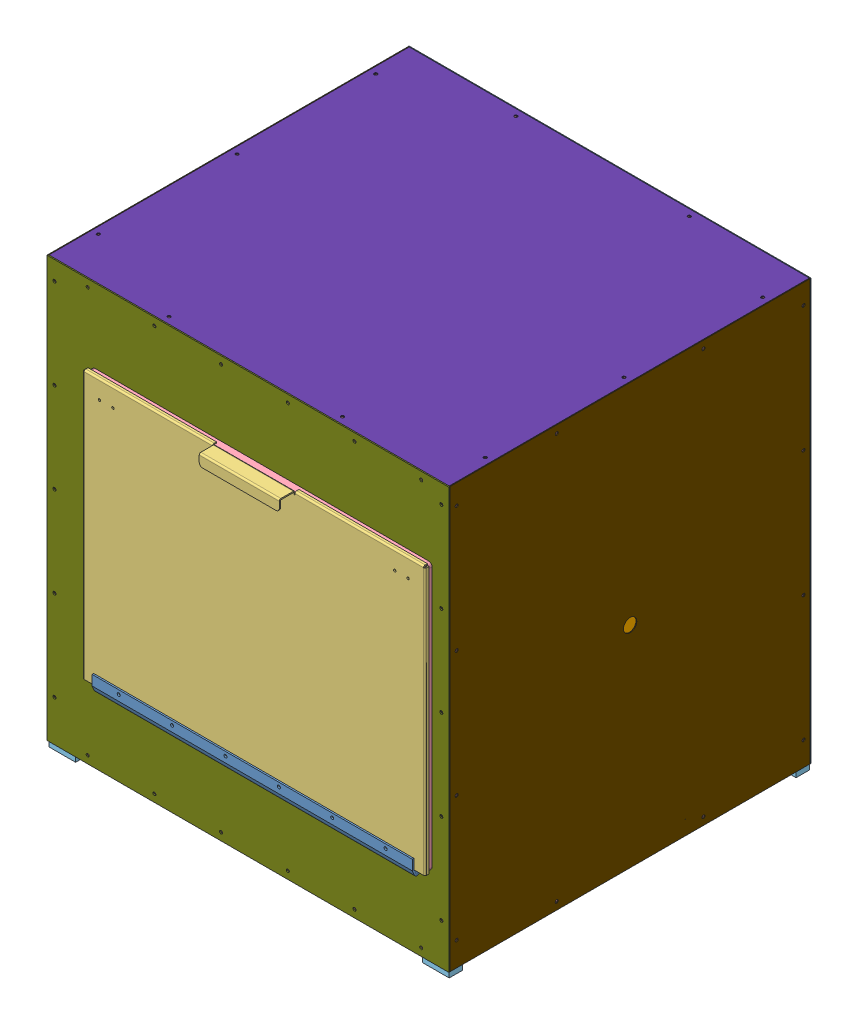
SolidWorks assembly Larva Tracker Assembly_Updated, configuration Default. Lengths in mm.
Overall size (765.17 811.21 817.56).
531 component instances, 63 part files, 154 mates.
Components (placement in the parent):
- T-LSR450-2: T-LSR450 [Default] at (-127.5387 61.5256 -39.6366) x (0 0 -1) z (1 0 0) size (65 43.34 637)
  - NM17-H-1: NM17-H [Default] at (-58.1732 -51.5031 48.5355) size (42.1 42.1 71.3)
  - T-NM17 Housing-1: T-NM17 Housing [Default] at (-16.1232 -51.2531 48.5355) x (-1 0 0) z (0 0 -1) size (41.8 41.8 52)
  - knob_LA-1: knob_LA [Default] at (-37.2232 -26.0531 -6.7645) (suppressed, hidden)
  - Coupling_CPS12-1: Coupling_CPS12 [Default] at (-37.0232 -30.3531 128.8355) x (0.334969 -0.942229 0) z (0 0 -1) size (12 12 14)
  - Car sub assy-1: Car sub assy [Default] at (-37.0232 -30.3531 234.0931) size (64 28.83 65.47) (suppressed, hidden)
    - Lead Screw Nut-1: Lead Screw Nut [Default] at origin size (22.86 20.6 25.4)
    - Screw_M3x12 CS-1: Screw_M3x12 CS [Default] at (8.2532 -4.765 4.546) size (5.92 5.92 12)
    - Screw_M3x12 CS-2: Screw_M3x12 CS [Default] at (-8.2532 -4.765 4.546) size (5.92 5.92 12)
    - Screw_M3x12 CS-3: Screw_M3x12 CS [Default] at (0 9.53 4.546) size (5.92 5.92 12)
    - Washer_5-32ID-1: Washer_5-32ID [Default] at (18.1354 5.1807 -52.75) x (0.633432 -0.633432 -0.44444) z (0.707107 0.707107 0) size (6.35 6.35 0.33)
    - Bearing Washer-1: Bearing Washer [Default] at (-18.3674 -8.3405 -0.25) x (0.5 -0.5 -0.707107) z (0.707107 0.707107 0) size (6.35 6.35 0.2)
    - 3%8 in bearing-1: 3%8 in bearing [Default] at (18.226 -8.199 -0.25) x (0.42856 0.42856 -0.795407) z (-0.707107 0.707107 0) size (9.53 9.53 3.17)
    - Bearing Washer-2: Bearing Washer [Default] at (15.9809 -5.954 -0.25) x (0.5 0.5 0.707107) z (-0.707107 0.707107 0) size (6.35 6.35 0.2)
    - Bearing Washer-3: Bearing Washer [Default] at (18.2273 5.2726 -8.75) x (0.5 -0.5 -0.707107) z (0.707107 0.707107 0) size (6.35 6.35 0.2)
    - 3%8 in bearing-2: 3%8 in bearing [Default] at (15.9822 3.0276 -8.75) x (0.5 -0.5 -0.707107) z (0.707107 0.707107 0) size (9.53 9.53 3.17)
    - 3%8 in bearing-3: 3%8 in bearing [Default] at (15.8903 2.9356 -52.75) x (0.65714 -0.65714 -0.369234) z (0.707107 0.707107 0) size (9.53 9.53 3.17)
    - ShoulderScrew-1: ShoulderScrew [Default] at (15.8903 2.9356 -52.75) x (0.530428 -0.530428 0.66128) z (-0.707107 -0.707107 0) size (7.95 7.95 13.65)
    - Bearing Washer-4: Bearing Washer [Default] at (15.9809 -5.954 -44.25) x (0.5 0.5 0.707107) z (-0.707107 0.707107 0) size (6.35 6.35 0.2)
    - 3%8 in bearing-4: 3%8 in bearing [Default] at (18.226 -8.199 -44.25) x (0.42856 0.42856 -0.795407) z (-0.707107 0.707107 0) size (9.53 9.53 3.17)
    - ShoulderScrew-2: ShoulderScrew [Default] at (18.226 -8.199 -44.25) x (0.405923 0.405923 -0.818812) z (0.707107 -0.707107 0) size (7.95 7.95 13.65)
    - ShoulderScrew-3: ShoulderScrew [Default] at (-18.226 -8.199 -44.25) x (0.498357 -0.498357 -0.709423) z (-0.707107 -0.707107 0) size (7.95 7.95 13.65)
    - ShoulderScrew-4: ShoulderScrew [Default] at (15.9822 3.0276 -8.75) x (0.496183 -0.496183 -0.712464) z (-0.707107 -0.707107 0) size (7.95 7.95 13.65)
    - Bearing Washer-5: Bearing Washer [Default] at (-15.9809 -5.954 -44.25) x (0.5 -0.5 -0.707107) z (0.707107 0.707107 0) size (6.35 6.35 0.2)
    - 3%8 in bearing-5: 3%8 in bearing [Default] at (-15.9809 -5.954 -44.25) x (-0.308196 0.308196 -0.900017) z (-0.707107 -0.707107 0) size (9.53 9.53 3.17)
    - Bearing Washer-6: Bearing Washer [Default] at (-18.3687 5.4141 -52.75) x (0.408741 0.408741 -0.816004) z (0.707107 -0.707107 0) size (6.35 6.35 0.2)
    - ShoulderScrew-5: ShoulderScrew [Default] at (-15.9822 3.0276 -52.75) x (0.451656 0.451656 -0.769424) z (0.707107 -0.707107 0) size (7.95 7.95 13.65)
    - 3%8 in bearing-6: 3%8 in bearing [Default] at (-18.2273 5.2726 -52.75) x (0.225478 0.225478 -0.947797) z (0.707107 -0.707107 0) size (9.53 9.53 3.17)
    - ShoulderScrew-6: ShoulderScrew [Default] at (18.226 -8.199 -0.25) x (0.471234 0.471234 -0.745572) z (0.707107 -0.707107 0) size (7.95 7.95 13.65)
    - Bearing Washer-7: Bearing Washer [Default] at (-15.9809 -5.954 -0.25) x (0.5 -0.5 -0.707107) z (0.707107 0.707107 0) size (6.35 6.35 0.2)
    - 3%8 in bearing-7: 3%8 in bearing [Default] at (-15.9809 -5.954 -0.25) x (-0.308196 0.308196 -0.900017) z (-0.707107 -0.707107 0) size (9.53 9.53 3.17)
    - Bearing Washer-8: Bearing Washer [Default] at (-18.2273 5.2726 -8.75) x (-0.44628 -0.44628 -0.775672) z (-0.707107 0.707107 0) size (6.35 6.35 0.2)
    - ShoulderScrew-7: ShoulderScrew [Default] at (-15.9822 3.0276 -8.75) x (-0.382714 -0.382714 -0.840868) z (0.707107 -0.707107 0) size (7.95 7.95 13.65)
    - 3%8 in bearing-8: 3%8 in bearing [Default] at (-18.2273 5.2726 -8.75) x (-0.663315 -0.663315 -0.34645) z (0.707107 -0.707107 0) size (9.53 9.53 3.17)
    - ShoulderScrew-8: ShoulderScrew [Default] at (-18.3674 -8.3405 -0.25) x (0.692139 -0.692139 0.204665) z (-0.707107 -0.707107 0) size (7.95 7.95 13.65)
    - T-LSR Top-1: T-LSR Top [Default] at (-23.2 -10.11 -59) size (64 23.75 65.05)
  - T-LSR450 Lead Screw-1: T-LSR450 Lead Screw [Default] at (-37.0232 -30.3507 123.8355) x (0.360518 -0.932752 0) z (0 0 1) size (6.34 6.34 506.7)
  - Screw M3 x 6 set screw-1: Screw M3 x 6 set screw [Default] at (-11.9381 -34.2188 486.5355) x (0.680208 0.680208 -0.273191) z (0.707107 -0.707107 0) size (3 3 6)
  - Screw M3 x 6 set screw-2: Screw M3 x 6 set screw [Default] at (-11.9381 -34.2188 461.5355) x (0.680208 0.680208 -0.273191) z (0.707107 -0.707107 0) size (3 3 6)
  - Screw M3 x 6 set screw-3: Screw M3 x 6 set screw [Default] at (-11.9381 -34.2188 436.5355) x (0.680208 0.680208 -0.273191) z (0.707107 -0.707107 0) size (3 3 6)
  - Screw M3 x 6 set screw-4: Screw M3 x 6 set screw [Default] at (-62.1082 -34.2188 461.5355) x (0.146534 -0.146534 0.978292) z (-0.707107 -0.707107 0) size (3 3 6)
  - Screw M3 x 6 set screw-5: Screw M3 x 6 set screw [Default] at (-62.1082 -34.2188 436.5355) x (0.289314 -0.289314 0.912466) z (-0.707107 -0.707107 0) size (3 3 6)
  - Screw M3 x 6 set screw-6: Screw M3 x 6 set screw [Default] at (-11.9381 -34.2188 536.5355) x (0.680208 0.680208 -0.273191) z (0.707107 -0.707107 0) size (3 3 6)
  - Screw M3 x 6 set screw-7: Screw M3 x 6 set screw [Default] at (-62.1082 -34.2188 411.5355) x (0.704993 -0.704993 0.077261) z (-0.707107 -0.707107 0) size (3 3 6)
  - Screw M3 x 6 set screw-8: Screw M3 x 6 set screw [Default] at (-11.9381 -34.2188 561.5355) x (0.680208 0.680208 -0.273191) z (0.707107 -0.707107 0) size (3 3 6)
  - Screw M3 x 6 set screw-9: Screw M3 x 6 set screw [Default] at (-11.9381 -34.2188 511.5355) x (0.680208 0.680208 -0.273191) z (0.707107 -0.707107 0) size (3 3 6)
  - Screw M3 x 6 set screw-10: Screw M3 x 6 set screw [Default] at (-62.1082 -34.2188 486.5355) x (0.67969 -0.67969 0.275758) z (-0.707107 -0.707107 0) size (3 3 6)
  - Screw M3 x 6 set screw-11: Screw M3 x 6 set screw [Default] at (-62.1082 -34.2188 511.5355) x (-0.395154 0.395154 -0.829281) z (-0.707107 -0.707107 0) size (3 3 6)
  - Screw M3 x 6 set screw-12: Screw M3 x 6 set screw [Default] at (-62.1082 -34.2188 561.5355) x (-0.551643 0.551643 -0.625603) z (-0.707107 -0.707107 0) size (3 3 6)
  - Screw M3 x 6 set screw-13: Screw M3 x 6 set screw [Default] at (-62.1082 -34.2188 536.5355) x (-0.617589 0.617589 -0.486998) z (-0.707107 -0.707107 0) size (3 3 6)
  - Screw M3 x 6 set screw-14: Screw M3 x 6 set screw [Default] at (-11.9381 -34.2188 586.5355) x (0.680208 0.680208 -0.273191) z (0.707107 -0.707107 0) size (3 3 6)
  - Screw M3 x 6 set screw-15: Screw M3 x 6 set screw [Default] at (-62.1082 -34.2188 611.5355) x (-0.585905 0.585905 -0.559849) z (-0.707107 -0.707107 0) size (3 3 6)
  - Screw M3 x 6 set screw-16: Screw M3 x 6 set screw [Default] at (-62.1082 -34.2188 586.5355) x (-0.690783 0.690783 -0.213627) z (-0.707107 -0.707107 0) size (3 3 6)
  - Screw M3 x 6 set screw-17: Screw M3 x 6 set screw [Default] at (-11.9381 -34.2188 611.5355) x (0.680208 0.680208 -0.273191) z (0.707107 -0.707107 0) size (3 3 6)
  - Screw M3 x 6 set screw-18: Screw M3 x 6 set screw [Default] at (-11.9381 -34.2188 411.5355) x (0.680208 0.680208 -0.273191) z (0.707107 -0.707107 0) size (3 3 6)
  - Bearing_Thrust_4-8-4-1: Bearing_Thrust_4-8-4 [Default] at (-37.0232 -30.3507 624.2355) size (9 9 4)
  - Bearing_Thrust_4-8-4-2: Bearing_Thrust_4-8-4 [Default] at (-37.0232 -30.3507 630.0355) size (9 9 4)
  - Screw_M3 x 5 Button Cap-1: Screw_M3 x 5 Button Cap [Default] at (-37.0232 -30.3507 631.3355) size (5.7 5.7 6.65)
  - T-LSR450 Base-1: T-LSR450 Base [Default] at (-69.5232 -52.7431 101.5355) size (65 27 520)
  - T-LSR450 Compression Bar-1: T-LSR450 Compression Bar [Default] at (-59.7393 -36.3047 101.5355) x (0.707107 0.707107 0) z (0 0 1) size (6.35 6.35 519.5)
  - T-LSR Bearing End Plate_Thrust Bearing Version1-1: T-LSR Bearing End Plate_Thrust Bearing Version1 [Default] at (-5.0232 -52.2431 633.5355) x (-1 0 0) z (0 0 -1) size (64 34.8 12)
  - Motor Mount End Plate-1: Motor Mount End Plate [Default] at (-69.0232 -52.2431 95.5355) size (64 42 6)
  - T-LSR450 Compression Bar-2: T-LSR450 Compression Bar [Default] at (-14.3071 -36.3047 101.5355) x (0.707107 0.707107 0) z (0 0 1) size (6.35 6.35 519.5)
  - Screw M3 x 8 SC-1: Screw M3 x 8 SC [Default] at (-8.5232 -48.7431 624.5355) size (5.5 5.5 11)
  - Screw M3 x 8 SC-2: Screw M3 x 8 SC [Default] at (-65.5232 -28.7431 624.5355) size (5.5 5.5 11)
  - Screw M3 x 8 SC-3: Screw M3 x 8 SC [Default] at (-8.5232 -28.7431 624.5355) size (5.5 5.5 11)
  - Screw M3 x 8 SC-4: Screw M3 x 8 SC [Default] at (-65.5232 -48.7431 624.5355) size (5.5 5.5 11)
  - Screw M3 x 8 SC-5: Screw M3 x 8 SC [Default] at (-21.5232 -14.8531 98.3355) size (5.5 5.5 11)
  - Screw M3 x 8 SC-6: Screw M3 x 8 SC [Default] at (-52.5232 -14.8531 98.3355) size (5.5 5.5 11)
  - Screw M3 x 8 SC-7: Screw M3 x 8 SC [Default] at (-21.5232 -45.8531 98.3355) size (5.5 5.5 11)
  - Screw M3 x 8 SC-8: Screw M3 x 8 SC [Default] at (-65.5232 -28.7431 98.5355) x (0.044892 0.998992 0) z (0 0 -1) size (5.5 5.5 11)
  - Screw M3 x 8 SC-9: Screw M3 x 8 SC [Default] at (-8.5232 -28.7431 98.5355) x (-0.436079 0.899908 0) z (0 0 -1) size (5.5 5.5 11)
  - Screw M3 x 8 SC-10: Screw M3 x 8 SC [Default] at (-8.5232 -48.7431 98.5355) x (0.383001 0.923748 0) z (0 0 -1) size (5.5 5.5 11)
  - Screw M3 x 8 SC-11: Screw M3 x 8 SC [Default] at (-65.5232 -48.7431 98.5355) x (0.453529 0.891241 0) z (0 0 -1) size (5.5 5.5 11)
  - Screw M3 x 8 SC-12: Screw M3 x 8 SC [Default] at (-52.5232 -45.8531 98.3355) size (5.5 5.5 11)
- Car sub assy-2: Car sub assy [Default] at (-20.0032 31.1749 -2.6134) x (0 0 1) z (-1 0 0) size (64 28.83 65.47)
  - Lead Screw Nut-1: Lead Screw Nut [Default] at origin size (22.86 20.6 25.4)
  - Screw_M3x12 CS-1: Screw_M3x12 CS [Default] at (8.2532 -4.765 4.546) size (5.92 5.92 12)
  - Screw_M3x12 CS-2: Screw_M3x12 CS [Default] at (-8.2532 -4.765 4.546) size (5.92 5.92 12)
  - Screw_M3x12 CS-3: Screw_M3x12 CS [Default] at (0 9.53 4.546) size (5.92 5.92 12)
  - Washer_5-32ID-1: Washer_5-32ID [Default] at (18.1354 5.1807 -52.75) x (0.633432 -0.633432 -0.44444) z (0.707107 0.707107 0) size (6.35 6.35 0.33)
  - Bearing Washer-1: Bearing Washer [Default] at (-18.3674 -8.3405 -0.25) x (0.5 -0.5 -0.707107) z (0.707107 0.707107 0) size (6.35 6.35 0.2)
  - 3%8 in bearing-1: 3%8 in bearing [Default] at (18.226 -8.199 -0.25) x (0.42856 0.42856 -0.795407) z (-0.707107 0.707107 0) size (9.53 9.53 3.17)
  - Bearing Washer-2: Bearing Washer [Default] at (15.9809 -5.954 -0.25) x (0.5 0.5 0.707107) z (-0.707107 0.707107 0) size (6.35 6.35 0.2)
  - Bearing Washer-3: Bearing Washer [Default] at (18.2273 5.2726 -8.75) x (0.5 -0.5 -0.707107) z (0.707107 0.707107 0) size (6.35 6.35 0.2)
  - 3%8 in bearing-2: 3%8 in bearing [Default] at (15.9822 3.0276 -8.75) x (0.5 -0.5 -0.707107) z (0.707107 0.707107 0) size (9.53 9.53 3.17)
  - 3%8 in bearing-3: 3%8 in bearing [Default] at (15.8903 2.9356 -52.75) x (0.65714 -0.65714 -0.369234) z (0.707107 0.707107 0) size (9.53 9.53 3.17)
  - ShoulderScrew-1: ShoulderScrew [Default] at (15.8903 2.9356 -52.75) x (0.530428 -0.530428 0.66128) z (-0.707107 -0.707107 0) size (7.95 7.95 13.65)
  - Bearing Washer-4: Bearing Washer [Default] at (15.9809 -5.954 -44.25) x (0.5 0.5 0.707107) z (-0.707107 0.707107 0) size (6.35 6.35 0.2)
  - 3%8 in bearing-4: 3%8 in bearing [Default] at (18.226 -8.199 -44.25) x (0.42856 0.42856 -0.795407) z (-0.707107 0.707107 0) size (9.53 9.53 3.17)
  - ShoulderScrew-2: ShoulderScrew [Default] at (18.226 -8.199 -44.25) x (0.405923 0.405923 -0.818812) z (0.707107 -0.707107 0) size (7.95 7.95 13.65)
  - ShoulderScrew-3: ShoulderScrew [Default] at (-18.226 -8.199 -44.25) x (0.498357 -0.498357 -0.709423) z (-0.707107 -0.707107 0) size (7.95 7.95 13.65)
  - ShoulderScrew-4: ShoulderScrew [Default] at (15.9822 3.0276 -8.75) x (0.496183 -0.496183 -0.712464) z (-0.707107 -0.707107 0) size (7.95 7.95 13.65)
  - Bearing Washer-5: Bearing Washer [Default] at (-15.9809 -5.954 -44.25) x (0.5 -0.5 -0.707107) z (0.707107 0.707107 0) size (6.35 6.35 0.2)
  - 3%8 in bearing-5: 3%8 in bearing [Default] at (-15.9809 -5.954 -44.25) x (-0.308196 0.308196 -0.900017) z (-0.707107 -0.707107 0) size (9.53 9.53 3.17)
  - Bearing Washer-6: Bearing Washer [Default] at (-18.3687 5.4141 -52.75) x (0.408741 0.408741 -0.816004) z (0.707107 -0.707107 0) size (6.35 6.35 0.2)
  - ShoulderScrew-5: ShoulderScrew [Default] at (-15.9822 3.0276 -52.75) x (0.451656 0.451656 -0.769424) z (0.707107 -0.707107 0) size (7.95 7.95 13.65)
  - 3%8 in bearing-6: 3%8 in bearing [Default] at (-18.2273 5.2726 -52.75) x (0.225478 0.225478 -0.947797) z (0.707107 -0.707107 0) size (9.53 9.53 3.17)
  - ShoulderScrew-6: ShoulderScrew [Default] at (18.226 -8.199 -0.25) x (0.471234 0.471234 -0.745572) z (0.707107 -0.707107 0) size (7.95 7.95 13.65)
  - Bearing Washer-7: Bearing Washer [Default] at (-15.9809 -5.954 -0.25) x (0.5 -0.5 -0.707107) z (0.707107 0.707107 0) size (6.35 6.35 0.2)
  - 3%8 in bearing-7: 3%8 in bearing [Default] at (-15.9809 -5.954 -0.25) x (-0.308196 0.308196 -0.900017) z (-0.707107 -0.707107 0) size (9.53 9.53 3.17)
  - Bearing Washer-8: Bearing Washer [Default] at (-18.2273 5.2726 -8.75) x (-0.44628 -0.44628 -0.775672) z (-0.707107 0.707107 0) size (6.35 6.35 0.2)
  - ShoulderScrew-7: ShoulderScrew [Default] at (-15.9822 3.0276 -8.75) x (-0.382714 -0.382714 -0.840868) z (0.707107 -0.707107 0) size (7.95 7.95 13.65)
  - 3%8 in bearing-8: 3%8 in bearing [Default] at (-18.2273 5.2726 -8.75) x (-0.663315 -0.663315 -0.34645) z (0.707107 -0.707107 0) size (9.53 9.53 3.17)
  - ShoulderScrew-8: ShoulderScrew [Default] at (-18.3674 -8.3405 -0.25) x (0.692139 -0.692139 0.204665) z (-0.707107 -0.707107 0) size (7.95 7.95 13.65)
  - T-LSR Top-1: T-LSR Top [Default] at (-23.2 -10.11 -59) size (64 23.75 65.05)
- Bottom Slider Bracket-1: Bottom Slider Bracket [Default] at (472.9968 -3 -2.6134) size (65 11.78 65)
- THK car-3: THK car [Default] at (482.5942 -27 267.3866) x (0 0 -1) z (1 0 0) size (60.5 19.5 34)
  - grease plug-1: grease plug [Default] at (540 0.1661 2.4399) x (-1 0 0) z (0 -0.135551 -0.99077) size (9.5 7.5 7.5)
  - THK SR-15W-1: THK SR-15W [Default] at origin size (57 19.5 34)
- THK Rail-1: THK Rail [Default] at (482.5942 -27 -254.1574) x (0 0 1) z (-1 0 0) size (538 12.5 15)
- LED Bracket-1: LED Bracket [Default] at (32.5868 44.5649 12.6266) x (0 0 1) z (-1 0 0) size (44.45 12.5 105.54)
- BL0202 Assy-1: BL0202 Assy [red] at (6.2016 57.0649 48.7454) x (0 0 -1) z (1 0 0) size (86.41 23.94 106.13)
  - BL020201-1: BL020201 [Default] at origin size (86.41 23.94 72.24)
  - BL Mounting Hardware-1: BL Mounting Hardware [Default] at (19.0531 4.4572 36.0096) x (-1 0 0) z (0 1 0) size (38.1 23.65 18.54)
  - BL Mounting Hardware-2: BL Mounting Hardware [Default] at (53.1845 4.4572 -36.0096) x (1 0 0) z (0 1 0) size (38.1 23.65 18.54)
- Glass plate assembly-1: Glass plate assembly [Default] at (232.1318 140.3134 -4.865) size (611.61 23.81 502.07)
  - Glass Plate-1: Glass Plate [Default] at origin size (475.4 9.53 475.4)
  - glass frame-1: glass frame [Default] x (-1 0 0) z (0 1 0) size (514.77 502.07 9.52)
  - label-1: label [Default] at (0 3.175 0) x (-1 0 0) z (0 1 0) size (101.6 9.52 2.54)
  - handle for glass plate-1: handle for glass plate [Default] at (251.035 8.7312 -50.8) x (0 0 1) z (-1 0 0) size (115.89 20.64 61.91)
  - handle for glass plate-2: handle for glass plate [Default] at (-251.035 8.7312 50.8) x (0 0 -1) z (1 0 0) size (115.89 20.64 61.91)
  - 5-16 24 nut mmc 94945A215-1: 5-16 24 nut mmc 94945A215 [94945A215] at (251.035 0 50.8) x (-0.5 0 -0.866025) z (-0.866025 0 0.5) size (12.7 6.6 14.66)
  - 5-16 24 nut mmc 94945A215-3: 5-16 24 nut mmc 94945A215 [94945A215] at (251.035 0 -50.8) x (-0.5 0 -0.866025) z (-0.866025 0 0.5) size (12.7 6.6 14.66)
  - 5-16 24 nut mmc 94945A215-4: 5-16 24 nut mmc 94945A215 [94945A215] at (-251.035 0 50.8) x (-0.50623 0.000007 0.862399) z (0.862399 0 0.50623) size (12.7 6.6 14.66)
  - 5-16 24 nut mmc 94945A215-5: 5-16 24 nut mmc 94945A215 [94945A215] at (-251.035 0 -50.8) x (-0.50623 0.000007 0.862399) z (0.862399 0 0.50623) size (12.7 6.6 14.66)
- Rail-1: Rail [Default] at (506.6618 121.2634 5.1974) size (41.27 22.23 685.8)
- Rail-2: Rail [Default] at (-42.3982 121.2634 5.1974) x (-1 0 0) z (0 0 -1) size (41.27 22.23 685.8)
- Camera and Lens-1: Camera and Lens [Default] at (6.2016 603.427 12.6266) x (0 1 0) z (-1 0 0) size (298.03 31.75 44)
  - Camera Body-1: Camera Body [Default] x (1 0 0) z (0 0 -1) size (73.22 29 44)
  - Lens Camera-1: Lens Camera [Default] at (-233.1136 0 0) x (0 0 -1) z (0 -1 0) size (31.75 230.07 31.75)
  - Camera Bracket_1-1: Camera Bracket_1 [Default] at (81.5205 49.265 0) x (0 0 -1) z (-1 0 0) (suppressed, hidden)
- T-LSR450-3: T-LSR450 [Default] at (-102.0264 419.4851 -420.5355) x (-1 0 0) z (0 0 1) size (65 43.34 637)
  - NM17-H-1: NM17-H [Default] at (-58.1732 -51.5031 48.5355) size (42.1 42.1 71.3)
  - T-NM17 Housing-1: T-NM17 Housing [Default] at (-16.1232 -51.2531 48.5355) x (-1 0 0) z (0 0 -1) size (41.8 41.8 52)
  - knob_LA-1: knob_LA [Default] at (-37.2232 -26.0531 -6.7645) (suppressed, hidden)
  - Coupling_CPS12-1: Coupling_CPS12 [Default] at (-37.0232 -30.3531 128.8355) x (0.334969 -0.942229 0) z (0 0 -1) size (12 12 14)
  - Car sub assy-1: Car sub assy [Default] at (-37.0232 -30.3531 234.0931) size (64 28.83 65.47) (suppressed, hidden)
    - Lead Screw Nut-1: Lead Screw Nut [Default] at origin size (22.86 20.6 25.4)
    - Screw_M3x12 CS-1: Screw_M3x12 CS [Default] at (8.2532 -4.765 4.546) size (5.92 5.92 12)
    - Screw_M3x12 CS-2: Screw_M3x12 CS [Default] at (-8.2532 -4.765 4.546) size (5.92 5.92 12)
    - Screw_M3x12 CS-3: Screw_M3x12 CS [Default] at (0 9.53 4.546) size (5.92 5.92 12)
    - Washer_5-32ID-1: Washer_5-32ID [Default] at (18.1354 5.1807 -52.75) x (0.633432 -0.633432 -0.44444) z (0.707107 0.707107 0) size (6.35 6.35 0.33)
    - Bearing Washer-1: Bearing Washer [Default] at (-18.3674 -8.3405 -0.25) x (0.5 -0.5 -0.707107) z (0.707107 0.707107 0) size (6.35 6.35 0.2)
    - 3%8 in bearing-1: 3%8 in bearing [Default] at (18.226 -8.199 -0.25) x (0.42856 0.42856 -0.795407) z (-0.707107 0.707107 0) size (9.53 9.53 3.17)
    - Bearing Washer-2: Bearing Washer [Default] at (15.9809 -5.954 -0.25) x (0.5 0.5 0.707107) z (-0.707107 0.707107 0) size (6.35 6.35 0.2)
    - Bearing Washer-3: Bearing Washer [Default] at (18.2273 5.2726 -8.75) x (0.5 -0.5 -0.707107) z (0.707107 0.707107 0) size (6.35 6.35 0.2)
    - 3%8 in bearing-2: 3%8 in bearing [Default] at (15.9822 3.0276 -8.75) x (0.5 -0.5 -0.707107) z (0.707107 0.707107 0) size (9.53 9.53 3.17)
    - 3%8 in bearing-3: 3%8 in bearing [Default] at (15.8903 2.9356 -52.75) x (0.65714 -0.65714 -0.369234) z (0.707107 0.707107 0) size (9.53 9.53 3.17)
    - ShoulderScrew-1: ShoulderScrew [Default] at (15.8903 2.9356 -52.75) x (0.530428 -0.530428 0.66128) z (-0.707107 -0.707107 0) size (7.95 7.95 13.65)
    - Bearing Washer-4: Bearing Washer [Default] at (15.9809 -5.954 -44.25) x (0.5 0.5 0.707107) z (-0.707107 0.707107 0) size (6.35 6.35 0.2)
    - 3%8 in bearing-4: 3%8 in bearing [Default] at (18.226 -8.199 -44.25) x (0.42856 0.42856 -0.795407) z (-0.707107 0.707107 0) size (9.53 9.53 3.17)
    - ShoulderScrew-2: ShoulderScrew [Default] at (18.226 -8.199 -44.25) x (0.405923 0.405923 -0.818812) z (0.707107 -0.707107 0) size (7.95 7.95 13.65)
    - ShoulderScrew-3: ShoulderScrew [Default] at (-18.226 -8.199 -44.25) x (0.498357 -0.498357 -0.709423) z (-0.707107 -0.707107 0) size (7.95 7.95 13.65)
    - ShoulderScrew-4: ShoulderScrew [Default] at (15.9822 3.0276 -8.75) x (0.496183 -0.496183 -0.712464) z (-0.707107 -0.707107 0) size (7.95 7.95 13.65)
    - Bearing Washer-5: Bearing Washer [Default] at (-15.9809 -5.954 -44.25) x (0.5 -0.5 -0.707107) z (0.707107 0.707107 0) size (6.35 6.35 0.2)
    - 3%8 in bearing-5: 3%8 in bearing [Default] at (-15.9809 -5.954 -44.25) x (-0.308196 0.308196 -0.900017) z (-0.707107 -0.707107 0) size (9.53 9.53 3.17)
    - Bearing Washer-6: Bearing Washer [Default] at (-18.3687 5.4141 -52.75) x (0.408741 0.408741 -0.816004) z (0.707107 -0.707107 0) size (6.35 6.35 0.2)
    - ShoulderScrew-5: ShoulderScrew [Default] at (-15.9822 3.0276 -52.75) x (0.451656 0.451656 -0.769424) z (0.707107 -0.707107 0) size (7.95 7.95 13.65)
    - 3%8 in bearing-6: 3%8 in bearing [Default] at (-18.2273 5.2726 -52.75) x (0.225478 0.225478 -0.947797) z (0.707107 -0.707107 0) size (9.53 9.53 3.17)
    - ShoulderScrew-6: ShoulderScrew [Default] at (18.226 -8.199 -0.25) x (0.471234 0.471234 -0.745572) z (0.707107 -0.707107 0) size (7.95 7.95 13.65)
    - Bearing Washer-7: Bearing Washer [Default] at (-15.9809 -5.954 -0.25) x (0.5 -0.5 -0.707107) z (0.707107 0.707107 0) size (6.35 6.35 0.2)
    - 3%8 in bearing-7: 3%8 in bearing [Default] at (-15.9809 -5.954 -0.25) x (-0.308196 0.308196 -0.900017) z (-0.707107 -0.707107 0) size (9.53 9.53 3.17)
    - Bearing Washer-8: Bearing Washer [Default] at (-18.2273 5.2726 -8.75) x (-0.44628 -0.44628 -0.775672) z (-0.707107 0.707107 0) size (6.35 6.35 0.2)
    - ShoulderScrew-7: ShoulderScrew [Default] at (-15.9822 3.0276 -8.75) x (-0.382714 -0.382714 -0.840868) z (0.707107 -0.707107 0) size (7.95 7.95 13.65)
    - 3%8 in bearing-8: 3%8 in bearing [Default] at (-18.2273 5.2726 -8.75) x (-0.663315 -0.663315 -0.34645) z (0.707107 -0.707107 0) size (9.53 9.53 3.17)
    - ShoulderScrew-8: ShoulderScrew [Default] at (-18.3674 -8.3405 -0.25) x (0.692139 -0.692139 0.204665) z (-0.707107 -0.707107 0) size (7.95 7.95 13.65)
    - T-LSR Top-1: T-LSR Top [Default] at (-23.2 -10.11 -59) size (64 23.75 65.05)
  - T-LSR450 Lead Screw-1: T-LSR450 Lead Screw [Default] at (-37.0232 -30.3507 123.8355) x (0.360518 -0.932752 0) z (0 0 1) size (6.34 6.34 506.7)
  - Screw M3 x 6 set screw-1: Screw M3 x 6 set screw [Default] at (-11.9381 -34.2188 486.5355) x (0.680208 0.680208 -0.273191) z (0.707107 -0.707107 0) size (3 3 6)
  - Screw M3 x 6 set screw-2: Screw M3 x 6 set screw [Default] at (-11.9381 -34.2188 461.5355) x (0.680208 0.680208 -0.273191) z (0.707107 -0.707107 0) size (3 3 6)
  - Screw M3 x 6 set screw-3: Screw M3 x 6 set screw [Default] at (-11.9381 -34.2188 436.5355) x (0.680208 0.680208 -0.273191) z (0.707107 -0.707107 0) size (3 3 6)
  - Screw M3 x 6 set screw-4: Screw M3 x 6 set screw [Default] at (-62.1082 -34.2188 461.5355) x (0.146534 -0.146534 0.978292) z (-0.707107 -0.707107 0) size (3 3 6)
  - Screw M3 x 6 set screw-5: Screw M3 x 6 set screw [Default] at (-62.1082 -34.2188 436.5355) x (0.289314 -0.289314 0.912466) z (-0.707107 -0.707107 0) size (3 3 6)
  - Screw M3 x 6 set screw-6: Screw M3 x 6 set screw [Default] at (-11.9381 -34.2188 536.5355) x (0.680208 0.680208 -0.273191) z (0.707107 -0.707107 0) size (3 3 6)
  - Screw M3 x 6 set screw-7: Screw M3 x 6 set screw [Default] at (-62.1082 -34.2188 411.5355) x (0.704993 -0.704993 0.077261) z (-0.707107 -0.707107 0) size (3 3 6)
  - Screw M3 x 6 set screw-8: Screw M3 x 6 set screw [Default] at (-11.9381 -34.2188 561.5355) x (0.680208 0.680208 -0.273191) z (0.707107 -0.707107 0) size (3 3 6)
  - Screw M3 x 6 set screw-9: Screw M3 x 6 set screw [Default] at (-11.9381 -34.2188 511.5355) x (0.680208 0.680208 -0.273191) z (0.707107 -0.707107 0) size (3 3 6)
  - Screw M3 x 6 set screw-10: Screw M3 x 6 set screw [Default] at (-62.1082 -34.2188 486.5355) x (0.67969 -0.67969 0.275758) z (-0.707107 -0.707107 0) size (3 3 6)
  - Screw M3 x 6 set screw-11: Screw M3 x 6 set screw [Default] at (-62.1082 -34.2188 511.5355) x (-0.395154 0.395154 -0.829281) z (-0.707107 -0.707107 0) size (3 3 6)
  - Screw M3 x 6 set screw-12: Screw M3 x 6 set screw [Default] at (-62.1082 -34.2188 561.5355) x (-0.551643 0.551643 -0.625603) z (-0.707107 -0.707107 0) size (3 3 6)
  - Screw M3 x 6 set screw-13: Screw M3 x 6 set screw [Default] at (-62.1082 -34.2188 536.5355) x (-0.617589 0.617589 -0.486998) z (-0.707107 -0.707107 0) size (3 3 6)
  - Screw M3 x 6 set screw-14: Screw M3 x 6 set screw [Default] at (-11.9381 -34.2188 586.5355) x (0.680208 0.680208 -0.273191) z (0.707107 -0.707107 0) size (3 3 6)
  - Screw M3 x 6 set screw-15: Screw M3 x 6 set screw [Default] at (-62.1082 -34.2188 611.5355) x (-0.585905 0.585905 -0.559849) z (-0.707107 -0.707107 0) size (3 3 6)
  - Screw M3 x 6 set screw-16: Screw M3 x 6 set screw [Default] at (-62.1082 -34.2188 586.5355) x (-0.690783 0.690783 -0.213627) z (-0.707107 -0.707107 0) size (3 3 6)
  - Screw M3 x 6 set screw-17: Screw M3 x 6 set screw [Default] at (-11.9381 -34.2188 611.5355) x (0.680208 0.680208 -0.273191) z (0.707107 -0.707107 0) size (3 3 6)
  - Screw M3 x 6 set screw-18: Screw M3 x 6 set screw [Default] at (-11.9381 -34.2188 411.5355) x (0.680208 0.680208 -0.273191) z (0.707107 -0.707107 0) size (3 3 6)
  - Bearing_Thrust_4-8-4-1: Bearing_Thrust_4-8-4 [Default] at (-37.0232 -30.3507 624.2355) size (9 9 4)
  - Bearing_Thrust_4-8-4-2: Bearing_Thrust_4-8-4 [Default] at (-37.0232 -30.3507 630.0355) size (9 9 4)
  - Screw_M3 x 5 Button Cap-1: Screw_M3 x 5 Button Cap [Default] at (-37.0232 -30.3507 631.3355) size (5.7 5.7 6.65)
  - T-LSR450 Base-1: T-LSR450 Base [Default] at (-69.5232 -52.7431 101.5355) size (65 27 520)
  - T-LSR450 Compression Bar-1: T-LSR450 Compression Bar [Default] at (-59.7393 -36.3047 101.5355) x (0.707107 0.707107 0) z (0 0 1) size (6.35 6.35 519.5)
  - T-LSR Bearing End Plate_Thrust Bearing Version1-1: T-LSR Bearing End Plate_Thrust Bearing Version1 [Default] at (-5.0232 -52.2431 633.5355) x (-1 0 0) z (0 0 -1) size (64 34.8 12)
  - Motor Mount End Plate-1: Motor Mount End Plate [Default] at (-69.0232 -52.2431 95.5355) size (64 42 6)
  - T-LSR450 Compression Bar-2: T-LSR450 Compression Bar [Default] at (-14.3071 -36.3047 101.5355) x (0.707107 0.707107 0) z (0 0 1) size (6.35 6.35 519.5)
  - Screw M3 x 8 SC-1: Screw M3 x 8 SC [Default] at (-8.5232 -48.7431 624.5355) size (5.5 5.5 11)
  - Screw M3 x 8 SC-2: Screw M3 x 8 SC [Default] at (-65.5232 -28.7431 624.5355) size (5.5 5.5 11)
  - Screw M3 x 8 SC-3: Screw M3 x 8 SC [Default] at (-8.5232 -28.7431 624.5355) size (5.5 5.5 11)
  - Screw M3 x 8 SC-4: Screw M3 x 8 SC [Default] at (-65.5232 -48.7431 624.5355) size (5.5 5.5 11)
  - Screw M3 x 8 SC-5: Screw M3 x 8 SC [Default] at (-21.5232 -14.8531 98.3355) size (5.5 5.5 11)
  - Screw M3 x 8 SC-6: Screw M3 x 8 SC [Default] at (-52.5232 -14.8531 98.3355) size (5.5 5.5 11)
  - Screw M3 x 8 SC-7: Screw M3 x 8 SC [Default] at (-21.5232 -45.8531 98.3355) size (5.5 5.5 11)
  - Screw M3 x 8 SC-8: Screw M3 x 8 SC [Default] at (-65.5232 -28.7431 98.5355) x (0.044892 0.998992 0) z (0 0 -1) size (5.5 5.5 11)
  - Screw M3 x 8 SC-9: Screw M3 x 8 SC [Default] at (-8.5232 -28.7431 98.5355) x (-0.436079 0.899908 0) z (0 0 -1) size (5.5 5.5 11)
  - Screw M3 x 8 SC-10: Screw M3 x 8 SC [Default] at (-8.5232 -48.7431 98.5355) x (0.383001 0.923748 0) z (0 0 -1) size (5.5 5.5 11)
  - Screw M3 x 8 SC-11: Screw M3 x 8 SC [Default] at (-65.5232 -48.7431 98.5355) x (0.453529 0.891241 0) z (0 0 -1) size (5.5 5.5 11)
  - Screw M3 x 8 SC-12: Screw M3 x 8 SC [Default] at (-52.5232 -45.8531 98.3355) size (5.5 5.5 11)
- Car sub assy-3: Car sub assy [Default] at (-65.0032 449.8358 -16.8734) x (-1 0 0) z (0 0 1) size (64 28.83 65.47)
  - Lead Screw Nut-1: Lead Screw Nut [Default] at origin size (22.86 20.6 25.4)
  - Screw_M3x12 CS-1: Screw_M3x12 CS [Default] at (8.2532 -4.765 4.546) size (5.92 5.92 12)
  - Screw_M3x12 CS-2: Screw_M3x12 CS [Default] at (-8.2532 -4.765 4.546) size (5.92 5.92 12)
  - Screw_M3x12 CS-3: Screw_M3x12 CS [Default] at (0 9.53 4.546) size (5.92 5.92 12)
  - Washer_5-32ID-1: Washer_5-32ID [Default] at (18.1354 5.1807 -52.75) x (0.633432 -0.633432 -0.44444) z (0.707107 0.707107 0) size (6.35 6.35 0.33)
  - Bearing Washer-1: Bearing Washer [Default] at (-18.3674 -8.3405 -0.25) x (0.5 -0.5 -0.707107) z (0.707107 0.707107 0) size (6.35 6.35 0.2)
  - 3%8 in bearing-1: 3%8 in bearing [Default] at (18.226 -8.199 -0.25) x (0.42856 0.42856 -0.795407) z (-0.707107 0.707107 0) size (9.53 9.53 3.17)
  - Bearing Washer-2: Bearing Washer [Default] at (15.9809 -5.954 -0.25) x (0.5 0.5 0.707107) z (-0.707107 0.707107 0) size (6.35 6.35 0.2)
  - Bearing Washer-3: Bearing Washer [Default] at (18.2273 5.2726 -8.75) x (0.5 -0.5 -0.707107) z (0.707107 0.707107 0) size (6.35 6.35 0.2)
  - 3%8 in bearing-2: 3%8 in bearing [Default] at (15.9822 3.0276 -8.75) x (0.5 -0.5 -0.707107) z (0.707107 0.707107 0) size (9.53 9.53 3.17)
  - 3%8 in bearing-3: 3%8 in bearing [Default] at (15.8903 2.9356 -52.75) x (0.65714 -0.65714 -0.369234) z (0.707107 0.707107 0) size (9.53 9.53 3.17)
  - ShoulderScrew-1: ShoulderScrew [Default] at (15.8903 2.9356 -52.75) x (0.530428 -0.530428 0.66128) z (-0.707107 -0.707107 0) size (7.95 7.95 13.65)
  - Bearing Washer-4: Bearing Washer [Default] at (15.9809 -5.954 -44.25) x (0.5 0.5 0.707107) z (-0.707107 0.707107 0) size (6.35 6.35 0.2)
  - 3%8 in bearing-4: 3%8 in bearing [Default] at (18.226 -8.199 -44.25) x (0.42856 0.42856 -0.795407) z (-0.707107 0.707107 0) size (9.53 9.53 3.17)
  - ShoulderScrew-2: ShoulderScrew [Default] at (18.226 -8.199 -44.25) x (0.405923 0.405923 -0.818812) z (0.707107 -0.707107 0) size (7.95 7.95 13.65)
  - ShoulderScrew-3: ShoulderScrew [Default] at (-18.226 -8.199 -44.25) x (0.498357 -0.498357 -0.709423) z (-0.707107 -0.707107 0) size (7.95 7.95 13.65)
  - ShoulderScrew-4: ShoulderScrew [Default] at (15.9822 3.0276 -8.75) x (0.496183 -0.496183 -0.712464) z (-0.707107 -0.707107 0) size (7.95 7.95 13.65)
  - Bearing Washer-5: Bearing Washer [Default] at (-15.9809 -5.954 -44.25) x (0.5 -0.5 -0.707107) z (0.707107 0.707107 0) size (6.35 6.35 0.2)
  - 3%8 in bearing-5: 3%8 in bearing [Default] at (-15.9809 -5.954 -44.25) x (-0.308196 0.308196 -0.900017) z (-0.707107 -0.707107 0) size (9.53 9.53 3.17)
  - Bearing Washer-6: Bearing Washer [Default] at (-18.3687 5.4141 -52.75) x (0.408741 0.408741 -0.816004) z (0.707107 -0.707107 0) size (6.35 6.35 0.2)
  - ShoulderScrew-5: ShoulderScrew [Default] at (-15.9822 3.0276 -52.75) x (0.451656 0.451656 -0.769424) z (0.707107 -0.707107 0) size (7.95 7.95 13.65)
  - 3%8 in bearing-6: 3%8 in bearing [Default] at (-18.2273 5.2726 -52.75) x (0.225478 0.225478 -0.947797) z (0.707107 -0.707107 0) size (9.53 9.53 3.17)
  - ShoulderScrew-6: ShoulderScrew [Default] at (18.226 -8.199 -0.25) x (0.471234 0.471234 -0.745572) z (0.707107 -0.707107 0) size (7.95 7.95 13.65)
  - Bearing Washer-7: Bearing Washer [Default] at (-15.9809 -5.954 -0.25) x (0.5 -0.5 -0.707107) z (0.707107 0.707107 0) size (6.35 6.35 0.2)
  - 3%8 in bearing-7: 3%8 in bearing [Default] at (-15.9809 -5.954 -0.25) x (-0.308196 0.308196 -0.900017) z (-0.707107 -0.707107 0) size (9.53 9.53 3.17)
  - Bearing Washer-8: Bearing Washer [Default] at (-18.2273 5.2726 -8.75) x (-0.44628 -0.44628 -0.775672) z (-0.707107 0.707107 0) size (6.35 6.35 0.2)
  - ShoulderScrew-7: ShoulderScrew [Default] at (-15.9822 3.0276 -8.75) x (-0.382714 -0.382714 -0.840868) z (0.707107 -0.707107 0) size (7.95 7.95 13.65)
  - 3%8 in bearing-8: 3%8 in bearing [Default] at (-18.2273 5.2726 -8.75) x (-0.663315 -0.663315 -0.34645) z (0.707107 -0.707107 0) size (9.53 9.53 3.17)
  - ShoulderScrew-8: ShoulderScrew [Default] at (-18.3674 -8.3405 -0.25) x (0.692139 -0.692139 0.204665) z (-0.707107 -0.707107 0) size (7.95 7.95 13.65)
  - T-LSR Top-1: T-LSR Top [Default] at (-23.2 -10.11 -59) size (64 23.75 65.05)
- T-LSR450-5: T-LSR450 [Default] at (-127.5387 377.3527 -6.3502) x (0 0 1) z (1 0 0) size (65 43.34 637)
  - NM17-H-1: NM17-H [Default] at (-58.1732 -51.5031 48.5355) size (42.1 42.1 71.3)
  - T-NM17 Housing-1: T-NM17 Housing [Default] at (-16.1232 -51.2531 48.5355) x (-1 0 0) z (0 0 -1) size (41.8 41.8 52)
  - knob_LA-1: knob_LA [Default] at (-37.2232 -26.0531 -6.7645) (suppressed, hidden)
  - Coupling_CPS12-1: Coupling_CPS12 [Default] at (-37.0232 -30.3531 128.8355) x (0.334969 -0.942229 0) z (0 0 -1) size (12 12 14)
  - Car sub assy-1: Car sub assy [Default] at (-37.0232 -30.3531 234.0931) size (64 28.83 65.47) (suppressed, hidden)
    - Lead Screw Nut-1: Lead Screw Nut [Default] at origin size (22.86 20.6 25.4)
    - Screw_M3x12 CS-1: Screw_M3x12 CS [Default] at (8.2532 -4.765 4.546) size (5.92 5.92 12)
    - Screw_M3x12 CS-2: Screw_M3x12 CS [Default] at (-8.2532 -4.765 4.546) size (5.92 5.92 12)
    - Screw_M3x12 CS-3: Screw_M3x12 CS [Default] at (0 9.53 4.546) size (5.92 5.92 12)
    - Washer_5-32ID-1: Washer_5-32ID [Default] at (18.1354 5.1807 -52.75) x (0.633432 -0.633432 -0.44444) z (0.707107 0.707107 0) size (6.35 6.35 0.33)
    - Bearing Washer-1: Bearing Washer [Default] at (-18.3674 -8.3405 -0.25) x (0.5 -0.5 -0.707107) z (0.707107 0.707107 0) size (6.35 6.35 0.2)
    - 3%8 in bearing-1: 3%8 in bearing [Default] at (18.226 -8.199 -0.25) x (0.42856 0.42856 -0.795407) z (-0.707107 0.707107 0) size (9.53 9.53 3.17)
    - Bearing Washer-2: Bearing Washer [Default] at (15.9809 -5.954 -0.25) x (0.5 0.5 0.707107) z (-0.707107 0.707107 0) size (6.35 6.35 0.2)
    - Bearing Washer-3: Bearing Washer [Default] at (18.2273 5.2726 -8.75) x (0.5 -0.5 -0.707107) z (0.707107 0.707107 0) size (6.35 6.35 0.2)
    - 3%8 in bearing-2: 3%8 in bearing [Default] at (15.9822 3.0276 -8.75) x (0.5 -0.5 -0.707107) z (0.707107 0.707107 0) size (9.53 9.53 3.17)
    - 3%8 in bearing-3: 3%8 in bearing [Default] at (15.8903 2.9356 -52.75) x (0.65714 -0.65714 -0.369234) z (0.707107 0.707107 0) size (9.53 9.53 3.17)
    - ShoulderScrew-1: ShoulderScrew [Default] at (15.8903 2.9356 -52.75) x (0.530428 -0.530428 0.66128) z (-0.707107 -0.707107 0) size (7.95 7.95 13.65)
    - Bearing Washer-4: Bearing Washer [Default] at (15.9809 -5.954 -44.25) x (0.5 0.5 0.707107) z (-0.707107 0.707107 0) size (6.35 6.35 0.2)
    - 3%8 in bearing-4: 3%8 in bearing [Default] at (18.226 -8.199 -44.25) x (0.42856 0.42856 -0.795407) z (-0.707107 0.707107 0) size (9.53 9.53 3.17)
    - ShoulderScrew-2: ShoulderScrew [Default] at (18.226 -8.199 -44.25) x (0.405923 0.405923 -0.818812) z (0.707107 -0.707107 0) size (7.95 7.95 13.65)
    - ShoulderScrew-3: ShoulderScrew [Default] at (-18.226 -8.199 -44.25) x (0.498357 -0.498357 -0.709423) z (-0.707107 -0.707107 0) size (7.95 7.95 13.65)
    - ShoulderScrew-4: ShoulderScrew [Default] at (15.9822 3.0276 -8.75) x (0.496183 -0.496183 -0.712464) z (-0.707107 -0.707107 0) size (7.95 7.95 13.65)
    - Bearing Washer-5: Bearing Washer [Default] at (-15.9809 -5.954 -44.25) x (0.5 -0.5 -0.707107) z (0.707107 0.707107 0) size (6.35 6.35 0.2)
    - 3%8 in bearing-5: 3%8 in bearing [Default] at (-15.9809 -5.954 -44.25) x (-0.308196 0.308196 -0.900017) z (-0.707107 -0.707107 0) size (9.53 9.53 3.17)
    - Bearing Washer-6: Bearing Washer [Default] at (-18.3687 5.4141 -52.75) x (0.408741 0.408741 -0.816004) z (0.707107 -0.707107 0) size (6.35 6.35 0.2)
    - ShoulderScrew-5: ShoulderScrew [Default] at (-15.9822 3.0276 -52.75) x (0.451656 0.451656 -0.769424) z (0.707107 -0.707107 0) size (7.95 7.95 13.65)
    - 3%8 in bearing-6: 3%8 in bearing [Default] at (-18.2273 5.2726 -52.75) x (0.225478 0.225478 -0.947797) z (0.707107 -0.707107 0) size (9.53 9.53 3.17)
    - ShoulderScrew-6: ShoulderScrew [Default] at (18.226 -8.199 -0.25) x (0.471234 0.471234 -0.745572) z (0.707107 -0.707107 0) size (7.95 7.95 13.65)
    - Bearing Washer-7: Bearing Washer [Default] at (-15.9809 -5.954 -0.25) x (0.5 -0.5 -0.707107) z (0.707107 0.707107 0) size (6.35 6.35 0.2)
    - 3%8 in bearing-7: 3%8 in bearing [Default] at (-15.9809 -5.954 -0.25) x (-0.308196 0.308196 -0.900017) z (-0.707107 -0.707107 0) size (9.53 9.53 3.17)
    - Bearing Washer-8: Bearing Washer [Default] at (-18.2273 5.2726 -8.75) x (-0.44628 -0.44628 -0.775672) z (-0.707107 0.707107 0) size (6.35 6.35 0.2)
    - ShoulderScrew-7: ShoulderScrew [Default] at (-15.9822 3.0276 -8.75) x (-0.382714 -0.382714 -0.840868) z (0.707107 -0.707107 0) size (7.95 7.95 13.65)
    - 3%8 in bearing-8: 3%8 in bearing [Default] at (-18.2273 5.2726 -8.75) x (-0.663315 -0.663315 -0.34645) z (0.707107 -0.707107 0) size (9.53 9.53 3.17)
    - ShoulderScrew-8: ShoulderScrew [Default] at (-18.3674 -8.3405 -0.25) x (0.692139 -0.692139 0.204665) z (-0.707107 -0.707107 0) size (7.95 7.95 13.65)
    - T-LSR Top-1: T-LSR Top [Default] at (-23.2 -10.11 -59) size (64 23.75 65.05)
  - T-LSR450 Lead Screw-1: T-LSR450 Lead Screw [Default] at (-37.0232 -30.3507 123.8355) x (0.360518 -0.932752 0) z (0 0 1) size (6.34 6.34 506.7)
  - Screw M3 x 6 set screw-1: Screw M3 x 6 set screw [Default] at (-11.9381 -34.2188 486.5355) x (0.680208 0.680208 -0.273191) z (0.707107 -0.707107 0) size (3 3 6)
  - Screw M3 x 6 set screw-2: Screw M3 x 6 set screw [Default] at (-11.9381 -34.2188 461.5355) x (0.680208 0.680208 -0.273191) z (0.707107 -0.707107 0) size (3 3 6)
  - Screw M3 x 6 set screw-3: Screw M3 x 6 set screw [Default] at (-11.9381 -34.2188 436.5355) x (0.680208 0.680208 -0.273191) z (0.707107 -0.707107 0) size (3 3 6)
  - Screw M3 x 6 set screw-4: Screw M3 x 6 set screw [Default] at (-62.1082 -34.2188 461.5355) x (0.146534 -0.146534 0.978292) z (-0.707107 -0.707107 0) size (3 3 6)
  - Screw M3 x 6 set screw-5: Screw M3 x 6 set screw [Default] at (-62.1082 -34.2188 436.5355) x (0.289314 -0.289314 0.912466) z (-0.707107 -0.707107 0) size (3 3 6)
  - Screw M3 x 6 set screw-6: Screw M3 x 6 set screw [Default] at (-11.9381 -34.2188 536.5355) x (0.680208 0.680208 -0.273191) z (0.707107 -0.707107 0) size (3 3 6)
  - Screw M3 x 6 set screw-7: Screw M3 x 6 set screw [Default] at (-62.1082 -34.2188 411.5355) x (0.704993 -0.704993 0.077261) z (-0.707107 -0.707107 0) size (3 3 6)
  - Screw M3 x 6 set screw-8: Screw M3 x 6 set screw [Default] at (-11.9381 -34.2188 561.5355) x (0.680208 0.680208 -0.273191) z (0.707107 -0.707107 0) size (3 3 6)
  - Screw M3 x 6 set screw-9: Screw M3 x 6 set screw [Default] at (-11.9381 -34.2188 511.5355) x (0.680208 0.680208 -0.273191) z (0.707107 -0.707107 0) size (3 3 6)
  - Screw M3 x 6 set screw-10: Screw M3 x 6 set screw [Default] at (-62.1082 -34.2188 486.5355) x (0.67969 -0.67969 0.275758) z (-0.707107 -0.707107 0) size (3 3 6)
  - Screw M3 x 6 set screw-11: Screw M3 x 6 set screw [Default] at (-62.1082 -34.2188 511.5355) x (-0.395154 0.395154 -0.829281) z (-0.707107 -0.707107 0) size (3 3 6)
  - Screw M3 x 6 set screw-12: Screw M3 x 6 set screw [Default] at (-62.1082 -34.2188 561.5355) x (-0.551643 0.551643 -0.625603) z (-0.707107 -0.707107 0) size (3 3 6)
  - Screw M3 x 6 set screw-13: Screw M3 x 6 set screw [Default] at (-62.1082 -34.2188 536.5355) x (-0.617589 0.617589 -0.486998) z (-0.707107 -0.707107 0) size (3 3 6)
  - Screw M3 x 6 set screw-14: Screw M3 x 6 set screw [Default] at (-11.9381 -34.2188 586.5355) x (0.680208 0.680208 -0.273191) z (0.707107 -0.707107 0) size (3 3 6)
  - Screw M3 x 6 set screw-15: Screw M3 x 6 set screw [Default] at (-62.1082 -34.2188 611.5355) x (-0.585905 0.585905 -0.559849) z (-0.707107 -0.707107 0) size (3 3 6)
  - Screw M3 x 6 set screw-16: Screw M3 x 6 set screw [Default] at (-62.1082 -34.2188 586.5355) x (-0.690783 0.690783 -0.213627) z (-0.707107 -0.707107 0) size (3 3 6)
  - Screw M3 x 6 set screw-17: Screw M3 x 6 set screw [Default] at (-11.9381 -34.2188 611.5355) x (0.680208 0.680208 -0.273191) z (0.707107 -0.707107 0) size (3 3 6)
  - Screw M3 x 6 set screw-18: Screw M3 x 6 set screw [Default] at (-11.9381 -34.2188 411.5355) x (0.680208 0.680208 -0.273191) z (0.707107 -0.707107 0) size (3 3 6)
